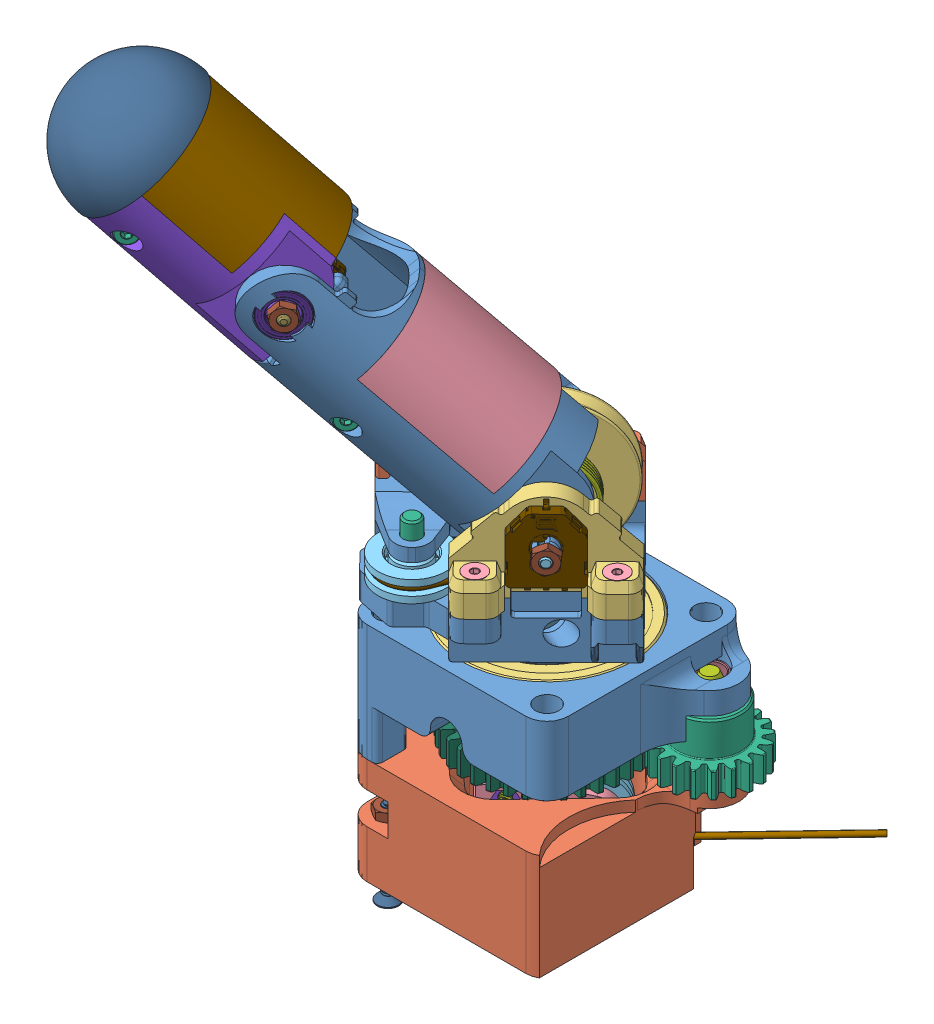
SolidWorks assembly mir-finger_subasm_pulley_rev21, configuration Default. Lengths in mm.
Overall size (131.1 142.98 100.14).
79 component instances, 44 part files, 24 mates.
Components (placement in the parent):
- mir-finger-base-module^mir-finger_subasm_pulley_rev21-1: mir-finger-base-module^mir-finger_subasm_pulley_rev21 [Default] at origin size (89.29 48.43 62.87) (virtual)
  - mir-finger_base_unlinked__rev2-1: mir-finger_base_unlinked__rev2 [Default] at origin size (89.29 22 38)
  - mir-finger_base_extend_rev2-1: mir-finger_base_extend_rev2 [Default] at (0 -20 0) x (-1 0 0) z (0 0 -1) size (59.5 28.31 62.87)
  - mir-finger_roll_joint_bearing_5972K157_rev2-1: mir-finger_roll_joint_bearing_5972K157_rev2 [5972K157] at (0 18.5 0) x (0 0 -1) z (0 1 0) size (32 32 7)
  - mir-guiding_pulley_asm_rev2-1: mir-guiding_pulley_asm_rev2 [Default] at (3.6839 -9.5 -3.8589) x (-0.690513 0 0.72332) z (0 -1 0) size (21.35 18.57 14)
    - mir-palm_pulley_support_rev2-1: mir-palm_pulley_support_rev2 [Default] at origin size (21.35 12 14)
    - mir-cable_guiding_pulley_3434T210_rev2-1: mir-cable_guiding_pulley_3434T210_rev2 [3434T21] at (0 0.1313 0) x (1 0 0) z (0 -1 0) size (12.7 12.7 4.76)
    - mir-cable_guiding_pulley_shaft_98105A085_rev2-1: mir-cable_guiding_pulley_shaft_98105A085_rev2 [98105A085] at (0 0.4375 0) x (0 -1 0) z (-0.873987 0 -0.48595) size (15.88 3.17 3.17)
    - mir-screw_guid_pulley_support_93395A150_rev2-1: mir-screw_guid_pulley_support_93395A150_rev2 [93395A150] at (11 11 -4) x (0.974914 0 -0.222582) z (0 -1 0) size (4 4 16.28)
    - mir-nut_guiding_pulley_m2_91828A111_rev2-1: mir-nut_guiding_pulley_m2_91828A111_rev2 [91828A111] at (11 -2.8 -4) x (0.866025 0 0.5) z (0 -1 0) size (4 4.62 1.83)
    - mir-nut_guiding_pulley_m2_91828A111_rev2-2: mir-nut_guiding_pulley_m2_91828A111_rev2 [91828A111] at (11 -2.8 4) x (0.866025 0 -0.5) z (0 -1 0) size (4 4.62 1.83)
    - mir-screw_guid_pulley_support_93395A150_rev2-2: mir-screw_guid_pulley_support_93395A150_rev2 [93395A150] at (11 11 4) x (0.974914 0 -0.222582) z (0 -1 0) size (4 4 16.28)
  - mir-finger_tendon_routing_lower_rev2-1: mir-finger_tendon_routing_lower_rev2 [Default] at (3.6839 -9.5 -3.8589) x (0.690513 0 -0.72332) z (0.72332 0 0.690513) size (45.86 11.22 1)
  - mir-screw_finger_base_extend_93395A150_rev2-1: mir-screw_finger_base_extend_93395A150_rev2 [93395A150] at (-15 -25 15) x (1 0 0) z (0 1 0) size (4 4 16.28)
  - mir-screw_finger_base_extend_93395A150_rev2-3: mir-screw_finger_base_extend_93395A150_rev2 [93395A150] at (-15 -25 -15) x (1 0 0) z (0 1 0) size (4 4 16.28)
  - mir-nut_M2_90591A265_rev21-2: mir-nut_M2_90591A265_rev21 [90591A265] at (-15 -10.2 -15) x (-0.866025 0 0.5) z (0 1 0) size (4 4.62 1.83)
  - mir-nut_M2_90591A265_rev21-3: mir-nut_M2_90591A265_rev21 [90591A265] at (-15 -10.2 15) x (1 0 0) z (0 1 0) size (4 4.62 1.83)
  - mir-screw_M2X25_91292A032_rev2-1: mir-screw_M2X25_91292A032_rev2 [91292A032] at (-15 -8 -15) x (1 0 0) z (0 1 0) size (3.8 3.8 27.16)
  - mir-screw_M2X25_91292A032_rev2-4: mir-screw_M2X25_91292A032_rev2 [91292A032] at (-15 -8 15) x (0 0 1) z (0 1 0) size (3.8 3.8 27.16)
  - mir-nut_M2_90591A265_rev21-4: mir-nut_M2_90591A265_rev21 [90591A265] at (-15 -5.8 15) x (0.866025 0 0.5) z (0 1 0) size (4 4.62 1.83)
  - mir-nut_M2_90591A265_rev21-5: mir-nut_M2_90591A265_rev21 [90591A265] at (-15 -5.8 -15) x (0.866025 0 0.5) z (0 1 0) size (4 4.62 1.83)
  - mir-finger_gear_bearing_57155K160_rev2-2: mir-finger_gear_bearing_57155K160_rev2 [57155K16] at (19.63 14.7875 -11) x (1 0 0) z (0 1 0) size (7.94 7.94 3.96)
  - mir-finger_gear_bearing_57155K160_rev2-3: mir-finger_gear_bearing_57155K160_rev2 [57155K16] at (19.63 -0.3125 -11) x (0.991858 0 -0.12735) z (0 1 0) size (7.94 7.94 3.96)
- mir-finger-roll-module^mir-finger_subasm_pulley_rev21-1: mir-finger-roll-module^mir-finger_subasm_pulley_rev21 [Default] at (0 43 0) x (0.700629 0 0.713526) z (-0.713526 0 0.700629) size (24 52.67 36.85) (virtual)
  - mir-cable_guiding_pulley_shaft_98105A085_rev2-1: mir-cable_guiding_pulley_shaft_98105A085_rev2 [98105A085] at (1.8594 -11.9375 18) x (0 -1 0) z (0 0 -1) size (15.88 3.17 3.17)
  - mir-cable_guiding_pulley_3434T210_rev2-1: mir-cable_guiding_pulley_3434T210_rev2 [3434T21] at (1.8594 -11.9812 18) x (0 0 -1) z (0 -1 0) size (12.7 12.7 4.76)
  - mir-horizontal-shaft-pulley^mir-finger-roll-module_mir-finger_subasm_pulley_rev21-1: mir-horizontal-shaft-pulley^mir-finger-roll-module_mir-finger_subasm_pulley_rev21 [Default] at (5.6117 -15.25 1.1374) x (0.392744 0 0.919648) z (-0.919648 0 0.392744) size (7.94 7.94 9.53) (virtual)
    - mir-finger_roll_pulley_bearing_57155k381_rev2-1: mir-finger_roll_pulley_bearing_57155k381_rev2 [57155K381] x (1 0 0) z (0 0 -1) size (7.94 7.94 4.37)
    - mir-finger_roll_pulley_shaft_98105A081_rev2-1: mir-finger_roll_pulley_shaft_98105A081_rev2 [98105A081] at (0 0 1.8104) x (0 0 -1) z (1 0 0) size (9.53 2.38 2.38)
    - mir-finger_shaft_pulley_custom_rev2-1: mir-finger_shaft_pulley_custom_rev2 [Default] at (0 0 4.6828) x (1 0 0) z (0 1 0) size (7.5 4 7.5)
  - mir-finger_joint_bearing_7804K104_rev2-1: mir-finger_joint_bearing_7804K104_rev2 [7804K104] at (-10.75 0 0) x (0 0 1) z (-1 0 0) size (8 8 2.5)
  - mir-finger_joint_bearing_7804K104_rev2-2: mir-finger_joint_bearing_7804K104_rev2 [7804K104] at (10.75 0 0) x (0 0 1) z (-1 0 0) size (8 8 2.5)
  - mir-finger_tendon_routing_rev2-1: mir-finger_tendon_routing_rev2 [Default] at (-3.6 0 0) x (0 0 1) z (-1 0 0) size (36.36 48.67 11.72)
- mir-finger-prox-module^mir-finger_subasm_pulley_rev21-1: mir-finger-prox-module^mir-finger_subasm_pulley_rev21 [Default] at (0.0486 43 0.0495) x (0.700629 0 0.713526) z (-0.50967 -0.699842 0.500457) size (32.29 69.16 25.33) (virtual)
  - mir-finger_prox_link_rev2-1: mir-finger_prox_link_rev2 [3d_printing] at origin size (29.2 74.5 29)
  - mir-finger_joint_bearing_7804K104_rev2-1: mir-finger_joint_bearing_7804K104_rev2 [7804K104] at (-2.75 0 0) x (0 0 1) z (-1 0 0) size (8 8 2.5)
  - mir-finger_prox_bushing_rev2-1: mir-finger_prox_bushing_rev2 [Default] at (-1.5 0 0) x (0 -1 0) z (0 0 1) size (6.7 1.5 6.7)
  - mir-finger_prox_pulley_rev2-1: mir-finger_prox_pulley_rev2 [Default] at (-5 0 0) x (1 0 0) z (0 1 0) size (4 25.66 25.33)
  - mir-finger_prox_rubber_rev2-1: mir-finger_prox_rubber_rev2 [Default] at (0 10 0) size (25 26 12.5)
  - mir-finger_joint_bearing_7804K104_rev2-2: mir-finger_joint_bearing_7804K104_rev2 [7804K104] at (10.75 50 0) x (0 0 1) z (-1 0 0) size (8 8 2.5)
  - mir-finger_joint_bearing_7804K104_rev2-3: mir-finger_joint_bearing_7804K104_rev2 [7804K104] at (-10.75 50 0) x (0 0 1) z (-1 0 0) size (8 8 2.5)
  - mir-91292A034_18-8 Stainless Steel Socket Head Screw_rev2-1: mir-91292A034_18-8 Stainless Steel Socket Head Screw_rev2 [91292A034] at (2.5 0 0) x (0 0 1) z (1 0 0) size (3.8 3.8 32.29)
  - mir-screw_M2X16_91292A002_rev2-1: mir-screw_M2X16_91292A002_rev2 [91292A002] at (-10 30 8) x (0 0 1) z (1 0 0) size (3.8 3.8 18.16)
  - mir-nut_M2_90591A265_rev21-1: mir-nut_M2_90591A265_rev21 [90591A265] at (-8.8 30 8) x (0 -0.866025 0.5) z (1 0 0) size (4 4.62 1.83)
  - mir-finger_prox_spring_LTL028E08S316_rev2-1: mir-finger_prox_spring_LTL028E08S316_rev2 [Default] at (5 0 0) x (0 0 -1) z (0 1 0) size (20.68 4.91 15.05)
- mir-finger-tip-module^mir-finger_subasm_pulley_rev21-1: mir-finger-tip-module^mir-finger_subasm_pulley_rev21 [Default] at (-24.9192 78.7149 24.566) x (0.700629 0 0.713526) z (-0.515722 -0.691078 0.5064) size (27.16 46.21 25.4) (virtual)
  - mir-finger_dist_link_rev2-1: mir-finger_dist_link_rev2 [Default] at origin size (25 36.17 25.31)
  - mir-finger_dist_rubber_rev2-1: mir-finger_dist_rubber_rev2 [Default] at origin size (25 27.5 12.5)
  - mir-finger_fingertip_rev2-1: mir-finger_fingertip_rev2 [Default] at (0 27.5 0) size (25.4 12.7 25.4)
  - mir-screw_M2X6_92290A013_rev2-1: mir-screw_M2X6_92290A013_rev2 [92290A013] at (-3.5 13 4.5) size (3.8 3.8 8.1)
  - mir-nut_M2_90591A265_rev21-1: mir-nut_M2_90591A265_rev21 [90591A265] at (-3.5 13 6.2) x (0.866025 0.5 0) z (0 0 1) size (4 4.62 1.83)
  - mir-screw_M2X16_91292A002_rev2-1: mir-screw_M2X16_91292A002_rev2 [91292A002] at (-10 22 8) x (0 0 -1) z (1 0 0) size (3.8 3.8 18.16)
  - mir-nut_M2_90591A265_rev21-2: mir-nut_M2_90591A265_rev21 [90591A265] at (-8.8 22 8) x (0 0.866025 -0.5) z (-1 0 0) size (4 4.62 1.83)
  - mir-screw_M2X25_91292A032_rev2-1: mir-screw_M2X25_91292A032_rev2 [91292A032] at (13.5 0 0) x (0 0 1) z (-1 0 0) size (3.8 3.8 27.16)
  - mir-nut_M2_90591A265_rev21-3: mir-nut_M2_90591A265_rev21 [90591A265] at (12.3 0 0) x (0 -1 0) z (1 0 0) size (4 4.62 1.83)
  - mir-finger_dist_spring_LTL018C08S316_rev2-1: mir-finger_dist_spring_LTL018C08S316_rev2 [Default] at (4 0 0) x (0 0 -1) z (0 -1 0) size (15.44 3.23 11.42)
- mir-90220A120_Vented Hex Head Screw_rev21-1: mir-90220A120_Vented Hex Head Screw_rev21 [90220A120] at (0 -2.2534 0) x (0.97034 0 -0.241744) z (0 1 0) size (11.11 12.83 23.49)
- mir-93365A160_Tapered Heat-Set Inserts for Plastic_rev21-1: mir-93365A160_Tapered Heat-Set Inserts for Plastic_rev21 [93365A160] at (0 13 0) x (-0.688871 0 0.724884) z (0.724884 0 0.688871) size (9.53 8.41 9.53)
- mir-finger_roll_gear_6832K550_rev21-1: mir-finger_roll_gear_6832K550_rev21 [6832K55] at (0 1.7153 0) x (-0.482459 0 0.875918) z (0 1 0) size (30.2 30.2 11.12)
- mir-91251A144_Black-Oxide Alloy Steel Socket Head Screw_rev21-1: mir-91251A144_Black-Oxide Alloy Steel Socket Head Screw_rev21 [91251A144] at (-2.2663 10.4778 -7.6782) x (0.951666 0.124229 -0.280891) z (0.283084 0 0.959095) size (5.74 5.74 10.31)
- Copy of Part1^mir-finger_subasm_pulley_rev21-1: Copy of Part1^mir-finger_subasm_pulley_rev21 [Default] at (0 6.4778 0) x (-0.718655 0 0.695366) z (0 -1 0) (virtual)
- mir-finger_roll_spacer_rev21-1: mir-finger_roll_spacer_rev21 [Default] at (0 6.4778 0) x (0.959095 0 -0.283084) z (0.283084 0 0.959095) size (26 8.52 26)
- mir-3382g-001-xxx_rev21-1: mir-3382g-001-xxx_rev21 [Default] at (-23.2852 78.2613 25.5958) x (0.50967 0.699842 -0.500457) z (-0.499356 0.714298 0.490329) size (11.16 3.52 14.9)
- mir-3382g-001-xxx_rev21-2: mir-3382g-001-xxx_rev21 [Default] at (9.1082 42.365 9.2758) x (-0.713526 0 0.700629) z (0 1 0) size (11.16 3.52 14.9)
- mir-nut_M2_90591A265_rev21-1: mir-nut_M2_90591A265_rev21 [90591A265] at (12.3096 43 12.5362) x (-0.708211 0.121832 0.695409) z (0.700629 0 0.713526) size (4 4.62 1.83)
- mir-finger_roll_base_assem_rev21-1: mir-finger_roll_base_assem_rev21 [Default] at (-26.8404 13.6277 3.3816) x (0.700629 0 0.713526) z (-0.713526 0 0.700629) size (36 42.5 38)
  - mir-finger_roll_base_rev2-1: mir-finger_roll_base_rev2 [3d_printing] at (16.3923 29.3723 -21.5206) size (44.74 42.5 66.76)
  - mir-finger_roll_base_leftwing_rev2-1: mir-finger_roll_base_leftwing_rev2 [3d_printing] at (16.3923 29.3723 -21.5206) size (52.45 42.25 66.76)
  - mir-finger_roll_base_rightwing_rev2-1: mir-finger_roll_base_rightwing_rev2 [3d_printing] at (16.3923 29.3723 -21.5206) size (45.79 42.25 66.76)
  - mir-92125A056_18-8 Stainless Steel Hex Drive Flat Head Screw_rev2-1: mir-92125A056_18-8 Stainless Steel Hex Drive Flat Head Screw_rev2 [92125A056] at (31.8923 20.9823 -12.0206) x (0.966943 0 0.254992) z (0 -1 0) size (4 4 10.24)
  - mir-90591A265_Zinc-Plated Steel Hex Nut_rev2-1: mir-90591A265_Zinc-Plated Steel Hex Nut_rev2 [90591A265] at (31.8923 16.5723 -12.0206) x (1 0 0) z (0 -1 0) size (4 4.62 1.87)
  - mir-90591A265_Zinc-Plated Steel Hex Nut_rev2-2: mir-90591A265_Zinc-Plated Steel Hex Nut_rev2 [90591A265] at (0.8923 16.5723 -12.0206) x (1 0 0) z (0 -1 0) size (4 4.62 1.87)
  - mir-90591A265_Zinc-Plated Steel Hex Nut_rev2-3: mir-90591A265_Zinc-Plated Steel Hex Nut_rev2 [90591A265] at (31.8923 16.5723 -31.0206) x (1 0 0) z (0 -1 0) size (4 4.62 1.87)
  - mir-90591A265_Zinc-Plated Steel Hex Nut_rev2-4: mir-90591A265_Zinc-Plated Steel Hex Nut_rev2 [90591A265] at (0.8923 16.5723 -31.0206) x (1 0 0) z (0 -1 0) size (4 4.62 1.87)
  - mir-92125A056_18-8 Stainless Steel Hex Drive Flat Head Screw_rev2-2: mir-92125A056_18-8 Stainless Steel Hex Drive Flat Head Screw_rev2 [92125A056] at (0.8923 20.9823 -12.0206) x (0.966943 0 0.254992) z (0 -1 0) size (4 4 10.24)
  - mir-92125A056_18-8 Stainless Steel Hex Drive Flat Head Screw_rev2-3: mir-92125A056_18-8 Stainless Steel Hex Drive Flat Head Screw_rev2 [92125A056] at (31.8923 20.9823 -31.0206) x (0.966943 0 0.254992) z (0 -1 0) size (4 4 10.24)
  - mir-92125A056_18-8 Stainless Steel Hex Drive Flat Head Screw_rev2-4: mir-92125A056_18-8 Stainless Steel Hex Drive Flat Head Screw_rev2 [92125A056] at (0.8923 20.9823 -31.0206) x (0.966943 0 0.254992) z (0 -1 0) size (4 4 10.24)
- finger_idler_gear_7880K290_rev2-1: finger_idler_gear_7880K290_rev2 [7880K29] at (19.63 1.7153 -11) x (-0.798363 0 -0.602177) z (0 -1 0) size (17.54 17.54 11.14)
- mir-finger_roll_idler_shaft-1: mir-finger_roll_idler_shaft [Default] at (19.63 -2.2313 -11) x (0.999961 0 0.008877) z (-0.008877 0 0.999961) size (4.76 19 4.76)
Mates (geometry in assembly coordinates):
- Coincident21: coincident aligned: plane of mir-finger-prox-module^mir-finger_subasm_pulley_rev21-1/mir-finger_prox_link_rev2-1 through (0.0486 43 0.0495) normal (0.700629 0 0.713526); plane of mir-finger-tip-module^mir-finger_subasm_pulley_rev21-1/mir-finger_dist_link_rev2-1 through (-24.9192 78.7149 24.566) normal (0.700629 0 0.713526)
- Coincident22: coincident aligned: plane of mir-finger-base-module^mir-finger_subasm_pulley_rev21-1 through (0 0 0) normal (0 0 1)
- Coincident23: coincident aligned: plane of mir-finger-base-module^mir-finger_subasm_pulley_rev21-1 through (0 0 0) normal (0 1 0)
- Coincident24: coincident aligned: plane of mir-finger-base-module^mir-finger_subasm_pulley_rev21-1 through (0 0 0) normal (1 0 0)
- Concentric13: concentric aligned: cylinder of mir-finger-roll-module^mir-finger_subasm_pulley_rev21-1/mir-finger_joint_bearing_7804K104_rev2-1 through (-6.656 43 -6.7785) axis (0.700629 0 0.713526) radius 2.5; cylinder of mir-finger-prox-module^mir-finger_subasm_pulley_rev21-1/mir-91292A034_18-8 Stainless Steel Socket Head Screw_rev2-1 through (13.0102 43 13.2497) axis (0.700629 0 0.713526) radius 1
- Concentric23: concentric aligned: cylinder of mir-91251A144_Black-Oxide Alloy Steel Socket Head Screw_rev21-1 through (-0.8714 10.4778 -2.9522) axis (0.283084 0 0.959095) radius 2.8702; cylinder of mir-finger_roll_spacer_rev21-1 through (-3.6801 10.4778 -12.4682) axis (0.283084 0 0.959095) radius 3.175
- Coincident25: coincident anti-aligned: plane of mir-finger_roll_gear_6832K550_rev21-1 through (0 6.4778 0) normal (0 1 0); plane of mir-finger_roll_spacer_rev21-1 through (0 6.4778 0) normal (0 -1 0)
- Coincident26: coincident anti-aligned: plane of mir-90220A120_Vented Hex Head Screw_rev21-1 through (-1.3432 1.7153 -5.3915) normal (0 1 0); plane of mir-finger_roll_gear_6832K550_rev21-1 through (0 1.7153 0) normal (0 -1 0)
- Concentric14: concentric aligned: circle of mir-3382g-001-xxx_rev21-1; cylinder of mir-finger-prox-module^mir-finger_subasm_pulley_rev21-1/mir-finger_prox_link_rev2-1 through (-16.5116 78.7149 33.1283) axis (-0.700629 0 -0.713526) radius 4.15
- Concentric15: concentric anti-aligned: cylinder of mir-finger-prox-module^mir-finger_subasm_pulley_rev21-1/mir-finger_prox_link_rev2-1 through (-2.7539 43 -2.8046) axis (-0.700629 0 -0.713526) radius 3; cylinder of mir-3382g-001-xxx_rev21-2 through (9.1794 43 9.3483) axis (0.700629 0 0.713526) radius 1.9939
- Parallel6: parallel aligned: plane of mir-finger-prox-module^mir-finger_subasm_pulley_rev21-1/mir-finger_prox_link_rev2-1 through (-33.2256 81.3089 32.7222) normal (-0.50967 -0.699842 0.500457); plane of mir-3382g-001-xxx_rev21-1 through (-26.0944 74.4039 28.3542) normal (-0.50967 -0.699842 0.500457)
- Concentric16: concentric aligned: circle of mir-finger-prox-module^mir-finger_subasm_pulley_rev21-1/mir-finger_prox_link_rev2-1; circle of mir-nut_M2_90591A265_rev21-1
- Coincident27: coincident anti-aligned: plane of mir-finger-prox-module^mir-finger_subasm_pulley_rev21-1/mir-finger_prox_link_rev2-1 through (11.7491 43 11.9654) normal (0.700629 0 0.713526); plane of mir-nut_M2_90591A265_rev21-1 through (13.0652 41.6102 10.6731) normal (-0.700629 0 -0.713526)
- Coincident28: coincident aligned: plane of mir-finger-tip-module^mir-finger_subasm_pulley_rev21-1/mir-finger_dist_link_rev2-1 through (-24.9192 78.7149 24.566) normal (-0.700629 0 -0.713526); plane of mir-3382g-001-xxx_rev21-1 through (-24.9192 78.7149 24.566) normal (-0.700629 0 -0.713526)
- Concentric17: concentric aligned: cylinder of mir-finger-roll-module^mir-finger_subasm_pulley_rev21-1/mir-finger_joint_bearing_7804K104_rev2-1 through (-6.656 43 -6.7785) axis (0.700629 0 0.713526) radius 3.0082; cylinder of mir-finger_roll_base_assem_rev21-1/mir-finger_roll_base_leftwing_rev2-1 through (-8.4075 43 -8.5623) axis (0.700629 0 0.713526) radius 4.15
- Concentric18: concentric anti-aligned: cylinder of mir-finger-base-module^mir-finger_subasm_pulley_rev21-1/mir-finger_roll_joint_bearing_5972K157_rev2-1 through (0 15 0) axis (0 -1 0) radius 10; cylinder of mir-finger_roll_base_assem_rev21-1/mir-finger_roll_base_rev2-1 through (0 17 0) axis (0 1 0) radius 9.9
- Coincident29: coincident anti-aligned: plane of mir-finger-base-module^mir-finger_subasm_pulley_rev21-1/mir-finger_roll_joint_bearing_5972K157_rev2-1 through (-10.35 22 0) normal (0 1 0); plane of mir-finger_roll_base_assem_rev21-1/mir-finger_roll_base_rev2-1 through (0 22 0) normal (0 -1 0)
- Coincident30: coincident anti-aligned: plane of mir-3382g-001-xxx_rev21-2 through (9.1082 42.365 9.2758) normal (-0.700629 0 -0.713526); plane of mir-finger_roll_base_assem_rev21-1/mir-finger_roll_base_rightwing_rev2-1 through (9.1082 43 9.2758) normal (0.700629 0 0.713526)
- Coincident32: coincident anti-aligned: plane of mir-finger-base-module^mir-finger_subasm_pulley_rev21-1/mir-finger_roll_joint_bearing_5972K157_rev2-1 through (-11.9011 15 0) normal (0 -1 0); plane of mir-finger_roll_spacer_rev21-1 through (0 15 0) normal (0 1 0)
- Concentric20: concentric anti-aligned: cylinder of mir-finger_roll_gear_6832K550_rev21-1 through (0 6.4778 0) axis (0 -1 0) radius 6.35; cylinder of mir-finger_roll_base_assem_rev21-1/mir-finger_roll_base_rev2-1 through (0 17 0) axis (0 1 0) radius 9.9
- Concentric21: concentric anti-aligned: cylinder of mir-finger_roll_spacer_rev21-1 through (0 15 0) axis (0 -1 0) radius 13; cylinder of mir-finger_roll_base_assem_rev21-1/mir-finger_roll_base_rev2-1 through (0 17 0) axis (0 1 0) radius 9.9
- Concentric24: concentric anti-aligned: cylinder of mir-finger-tip-module^mir-finger_subasm_pulley_rev21-1/mir-finger_dist_link_rev2-1 through (-24.9192 78.7149 24.566) axis (0.700629 0 0.713526) radius 2; cylinder of mir-3382g-001-xxx_rev21-1 through (-23.6735 78.7149 25.8346) axis (-0.700629 0 -0.713526) radius 1.9939
- Concentric25: concentric anti-aligned: cylinder of mir-finger-roll-module^mir-finger_subasm_pulley_rev21-1/mir-cable_guiding_pulley_shaft_98105A085_rev2-1 through (-11.5407 39 13.938) axis (0 -1 0) radius 1.5875; cylinder of mir-finger_roll_base_assem_rev21-1/mir-finger_roll_base_rev2-1 through (-11.5407 26 13.938) axis (0 1 0) radius 1.69
- Distance1: distance = 9.5694 mm anti-aligned: plane of mir-finger-prox-module^mir-finger_subasm_pulley_rev21-1/mir-finger_prox_link_rev2-1 through (0.0486 43 0.0495) normal (-0.700629 0 -0.713526); plane of mir-finger_roll_base_assem_rev21-1/mir-finger_roll_base_leftwing_rev2-1 through (-15.9318 28 2.3297) normal (0.700629 0 0.713526)
